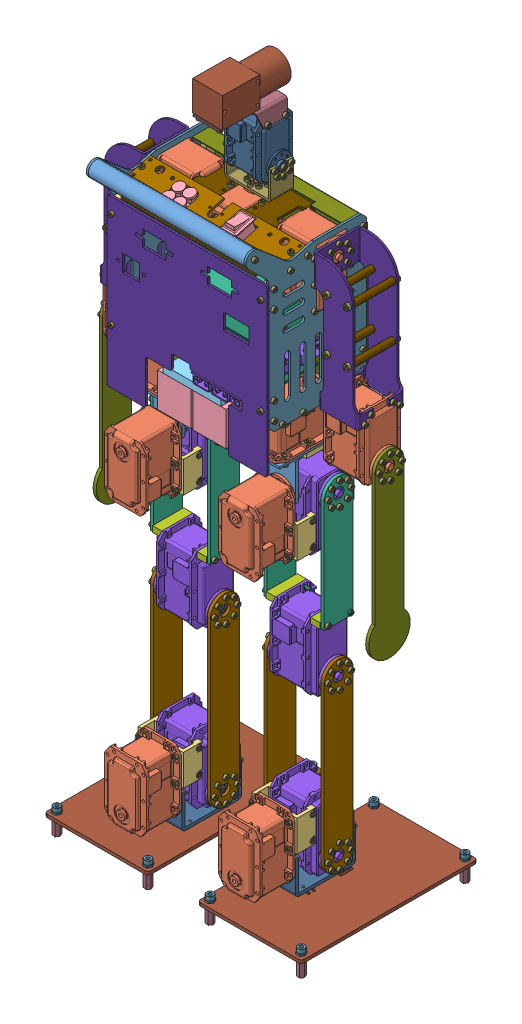
SolidWorks assembly 机器人, configuration 默认. Lengths in mm. (continued)
Components (placement in the parent): (continued)
- 躯干-1: 躯干 [默认] at (1014.3063 415.9938 -67.5657) size (172 287.24 163.85) (continued)
  - hexagon socket head cap screws gb-80: hexagon socket head cap screws gb [GB_FASTENER_SCREWS_HSHCS M2.5X6-N] at (86.3339 35.9855 124.55) x (0 1 0) z (0 0 1) size (8.5 4.5 4.5)
  - hexagon socket head cap screws gb-81: hexagon socket head cap screws gb [GB_FASTENER_SCREWS_HSHCS M2.5X6-N] at (-58.0661 35.9855 124.55) x (0 1 0) z (0 0 1) size (8.5 4.5 4.5)
  - hexagon socket head cap screws gb-82: hexagon socket head cap screws gb [GB_FASTENER_SCREWS_HSHCS M2.5X6-N] at (-58.0661 35.9855 146.55) x (0 1 0) z (0 0 1) size (8.5 4.5 4.5)
  - hexagon socket head cap screws gb-83: hexagon socket head cap screws gb [GB_FASTENER_SCREWS_HSHCS M2.5X6-N] at (-58.0661 35.9855 168.55) x (0 1 0) z (0 0 1) size (8.5 4.5 4.5)
  - hexagon socket head cap screws gb-84: hexagon socket head cap screws gb [GB_FASTENER_SCREWS_HSHCS M2.5X6-N] at (-58.0661 11.9855 124.55) x (0 -1 0) z (0 0 1) size (8.5 4.5 4.5)
  - hexagon socket head cap screws gb-85: hexagon socket head cap screws gb [GB_FASTENER_SCREWS_HSHCS M2.5X6-N] at (-58.0661 11.9855 146.55) x (0 -1 0) z (0 0 1) size (8.5 4.5 4.5)
  - hexagon socket head cap screws gb-86: hexagon socket head cap screws gb [GB_FASTENER_SCREWS_HSHCS M2.5X6-N] at (-58.0661 2.4855 168.55) x (0 1 0) z (0 0 1) size (8.5 4.5 4.5)
  - hexagon socket head cap screws gb-87: hexagon socket head cap screws gb [GB_FASTENER_SCREWS_HSHCS M2.5X6-N] at (-23.4661 2.4855 168.55) x (0 1 0) z (0 0 1) size (8.5 4.5 4.5)
  - hexagon socket head cap screws gb-89: hexagon socket head cap screws gb [GB_FASTENER_SCREWS_HSHCS M2.5X6-N] at (86.3339 11.9855 146.55) x (0 -1 0) z (0 0 1) size (8.5 4.5 4.5)
  - hexagon socket head cap screws gb-90: hexagon socket head cap screws gb [GB_FASTENER_SCREWS_HSHCS M2.5X6-N] at (86.3339 117.6114 168.55) x (0 -1 0) z (0 0 1) size (8.5 4.5 4.5)
  - hexagon socket head cap screws gb-91: hexagon socket head cap screws gb [GB_FASTENER_SCREWS_HSHCS M2.5X6-N] at (86.3339 2.4855 168.55) x (0 1 0) z (0 0 1) size (8.5 4.5 4.5)
  - hexagon socket head cap screws gb-92: hexagon socket head cap screws gb [GB_FASTENER_SCREWS_HSHCS M2.5X6-N] at (-23.4661 11.9855 124.55) x (0 -1 0) z (0 0 1) size (8.5 4.5 4.5)
  - hexagon socket head cap screws gb-93: hexagon socket head cap screws gb [GB_FASTENER_SCREWS_HSHCS M2.5X6-N] at (-23.4661 11.9855 146.55) x (0 -1 0) z (0 0 1) size (8.5 4.5 4.5)
  - hexagon socket head cap screws gb-94: hexagon socket head cap screws gb [GB_FASTENER_SCREWS_HSHCS M2.5X6-N] at (51.7339 11.9855 124.55) x (0 -1 0) z (0 0 1) size (8.5 4.5 4.5)
  - hexagon socket head cap screws gb-95: hexagon socket head cap screws gb [GB_FASTENER_SCREWS_HSHCS M2.5X6-N] at (51.7339 11.9855 146.55) x (0 -1 0) z (0 0 1) size (8.5 4.5 4.5)
  - hexagon socket head cap screws gb-96: hexagon socket head cap screws gb [GB_FASTENER_SCREWS_HSHCS M2.5X6-N] at (50.6339 166.8855 111.25) size (8.5 4.5 4.5)
  - hexagon socket head cap screws gb-97: hexagon socket head cap screws gb [GB_FASTENER_SCREWS_HSHCS M2.5X6-N] at (29.1612 177.7582 116.85) x (0 -1 0) z (0 0 1) size (8.5 4.5 4.5)
  - hexagon socket head cap screws gb-98: hexagon socket head cap screws gb [GB_FASTENER_SCREWS_HSHCS M2.5X6-N] at (-0.8934 177.7582 116.85) x (0 -1 0) z (0 0 1) size (8.5 4.5 4.5)
  - hexagon socket head cap screws gb-99: hexagon socket head cap screws gb [GB_FASTENER_SCREWS_HSHCS M2.5X6-N] at (-22.3661 166.8855 111.25) x (-1 0 0) z (0 0.924225 0.381849) size (8.5 4.5 4.5)
  - hexagon socket head cap screws gb-100: hexagon socket head cap screws gb [GB_FASTENER_SCREWS_HSHCS M2.5X6-N] at (14.1066 184.3582 121.35) x (0 -1 0) z (0 0 1) size (8.5 4.5 4.5)
  - hexagon socket head cap screws gb-101: hexagon socket head cap screws gb [GB_FASTENER_SCREWS_HSHCS M2.5X6-N] at (39.8284 204.3809 121.564) x (-0.999965 0 -0.008321) z (0.008321 0 -0.999965) size (8.5 4.5 4.5)
  - hexagon socket head cap screws gb-102: hexagon socket head cap screws gb [GB_FASTENER_SCREWS_HSHCS M2.5X6-N] at (-8.6199 204.3809 121.1609) x (0.999965 0 0.008321) z (-0.008321 0 0.999965) size (8.5 4.5 4.5)
  - hexagon socket head cap screws gb-103: hexagon socket head cap screws gb [GB_FASTENER_SCREWS_HSHCS M2.5X6-N] at (-0.8934 177.7582 133.85) x (0 -1 0) z (0 0 1) size (8.5 4.5 4.5)
  - hexagon socket head cap screws gb-104: hexagon socket head cap screws gb [GB_FASTENER_SCREWS_HSHCS M2.5X6-N] at (-22.3661 166.8855 145.85) x (-1 0 0) z (0 0.924225 0.381849) size (8.5 4.5 4.5)
  - hexagon socket head cap screws gb-105: hexagon socket head cap screws gb [GB_FASTENER_SCREWS_HSHCS M2.5X6-N] at (50.6339 166.8855 145.85) size (8.5 4.5 4.5)
  - hexagon socket head cap screws gb-106: hexagon socket head cap screws gb [GB_FASTENER_SCREWS_HSHCS M2.5X6-N] at (29.1612 177.7582 133.85) x (0 -1 0) z (0 0 1) size (8.5 4.5 4.5)
  - hexagon socket head cap screws gb-107: hexagon socket head cap screws gb [GB_FASTENER_SCREWS_HSHCS M2.5X6-N] at (8.497 183.5082 115.6463) x (0 -1 0) z (0 0 1) size (8.5 4.5 4.5)
  - hexagon socket head cap screws gb-108: hexagon socket head cap screws gb [GB_FASTENER_SCREWS_HSHCS M2.5X6-N] at (6.1069 183.5082 121.2834) x (0 -1 0) z (0 0 1) size (8.5 4.5 4.5)
  - hexagon socket head cap screws gb-109: hexagon socket head cap screws gb [GB_FASTENER_SCREWS_HSHCS M2.5X6-N] at (8.4029 183.5082 126.9596) x (0 -1 0) z (0 0 1) size (8.5 4.5 4.5)
  - hexagon socket head cap screws gb-110: hexagon socket head cap screws gb [GB_FASTENER_SCREWS_HSHCS M2.5X6-N] at (14.04 183.5082 129.3497) x (0 -1 0) z (0 0 1) size (8.5 4.5 4.5)
  - hexagon socket head cap screws gb-111: hexagon socket head cap screws gb [GB_FASTENER_SCREWS_HSHCS M2.5X6-N] at (19.7162 183.5082 127.0537) x (0 -1 0) z (0 0 1) size (8.5 4.5 4.5)
  - hexagon socket head cap screws gb-112: hexagon socket head cap screws gb [GB_FASTENER_SCREWS_HSHCS M2.5X6-N] at (22.1063 183.5082 121.4166) x (0 -1 0) z (0 0 1) size (8.5 4.5 4.5)
  - hexagon socket head cap screws gb-113: hexagon socket head cap screws gb [GB_FASTENER_SCREWS_HSHCS M2.5X6-N] at (19.8103 183.5082 115.7404) x (0 -1 0) z (0 0 1) size (8.5 4.5 4.5)
  - hexagon socket head cap screws gb-114: hexagon socket head cap screws gb [GB_FASTENER_SCREWS_HSHCS M2.5X6-N] at (14.1732 183.5082 113.3503) x (0 -1 0) z (0 0 1) size (8.5 4.5 4.5)
  - hexagon socket head cap screws gb-115: hexagon socket head cap screws gb [GB_FASTENER_SCREWS_HSHCS M2.5X6-N] at (93.6339 194.6934 203.5985) x (-1 0 0) z (0 0.924225 0.381849) size (8.5 4.5 4.5)
  - hexagon socket head cap screws gb-116: hexagon socket head cap screws gb [GB_FASTENER_SCREWS_HSHCS M2.5X6-N] at (-65.3661 194.6934 203.5985) size (8.5 4.5 4.5)
  - hexagon socket head cap screws gb-117: hexagon socket head cap screws gb [GB_FASTENER_SCREWS_HSHCS M2.5X6-N] at (23.6707 250.2249 136.7301) x (0 1 0) z (-0.004657 0 0.999989) size (8.5 4.5 4.5)
  - hexagon socket head cap screws gb-118: hexagon socket head cap screws gb [GB_FASTENER_SCREWS_HSHCS M2.5X6-N] at (3.6713 250.2249 136.5637) x (0 1 0) z (-0.004657 0 0.999989) size (8.5 4.5 4.5)
  - hexagon socket head cap screws gb-119: hexagon socket head cap screws gb [GB_FASTENER_SCREWS_HSHCS M2.5X6-N] at (3.4076 250.2249 168.2626) x (0 1 0) z (-0.004657 0 0.999989) size (8.5 4.5 4.5)
  - hexagon socket head cap screws gb-120: hexagon socket head cap screws gb [GB_FASTENER_SCREWS_HSHCS M2.5X6-N] at (23.4069 250.2249 168.429) x (0 1 0) z (-0.004657 0 0.999989) size (8.5 4.5 4.5)
  - Back-1: Back [默认] at (14.1339 170.328 166.311) x (1 0 0) z (0 0.965926 0.258819) size (100 30 26.32)
- hexagon socket head cap screws gb-1: hexagon socket head cap screws gb [GB_FASTENER_SCREWS_HSHCS M2.5X6-N] at (1114.4402 589.8793 60.9843) x (-1 0 0) z (0 0.924225 0.381849) size (8.5 4.5 4.5)
- hexagon socket head cap screws gb-2: hexagon socket head cap screws gb [GB_FASTENER_SCREWS_HSHCS M2.5X6-N] at (1114.4402 586.6575 53.2061) x (-1 0 0) z (0 0.924225 0.381849) size (8.5 4.5 4.5)
- hexagon socket head cap screws gb-3: hexagon socket head cap screws gb [GB_FASTENER_SCREWS_HSHCS M2.5X6-N] at (1114.4402 578.8793 49.9843) x (-1 0 0) z (0 0.924225 0.381849) size (8.5 4.5 4.5)
- hexagon socket head cap screws gb-4: hexagon socket head cap screws gb [GB_FASTENER_SCREWS_HSHCS M2.5X6-N] at (1114.4402 571.1012 53.2061) x (-1 0 0) z (0 0.924225 0.381849) size (8.5 4.5 4.5)
- hexagon socket head cap screws gb-5: hexagon socket head cap screws gb [GB_FASTENER_SCREWS_HSHCS M2.5X6-N] at (1114.4402 567.8793 60.9843) x (-1 0 0) z (0 0.924225 0.381849) size (8.5 4.5 4.5)
- hexagon socket head cap screws gb-6: hexagon socket head cap screws gb [GB_FASTENER_SCREWS_HSHCS M2.5X6-N] at (1114.4402 571.1012 68.7625) x (-1 0 0) z (0 0.924225 0.381849) size (8.5 4.5 4.5)
- hexagon socket head cap screws gb-7: hexagon socket head cap screws gb [GB_FASTENER_SCREWS_HSHCS M2.5X6-N] at (1114.4402 578.8793 71.9843) x (-1 0 0) z (0 0.924225 0.381849) size (8.5 4.5 4.5)
- hexagon socket head cap screws gb-8: hexagon socket head cap screws gb [GB_FASTENER_SCREWS_HSHCS M2.5X6-N] at (1114.4402 586.6575 68.7625) x (-1 0 0) z (0 0.924225 0.381849) size (8.5 4.5 4.5)
- hexagon socket head cap screws gb-25: hexagon socket head cap screws gb [GB_FASTENER_SCREWS_HSHCS M2.5X6-N] at (942.4402 586.6575 68.7625) size (8.5 4.5 4.5)
- hexagon socket head cap screws gb-26: hexagon socket head cap screws gb [GB_FASTENER_SCREWS_HSHCS M2.5X6-N] at (942.4402 578.8793 71.9843) size (8.5 4.5 4.5)
- hexagon socket head cap screws gb-27: hexagon socket head cap screws gb [GB_FASTENER_SCREWS_HSHCS M2.5X6-N] at (942.4402 571.1012 68.7625) size (8.5 4.5 4.5)
- hexagon socket head cap screws gb-28: hexagon socket head cap screws gb [GB_FASTENER_SCREWS_HSHCS M2.5X6-N] at (942.4402 567.8793 60.9843) size (8.5 4.5 4.5)
- hexagon socket head cap screws gb-29: hexagon socket head cap screws gb [GB_FASTENER_SCREWS_HSHCS M2.5X6-N] at (942.4402 589.8793 60.9843) size (8.5 4.5 4.5)
- hexagon socket head cap screws gb-30: hexagon socket head cap screws gb [GB_FASTENER_SCREWS_HSHCS M2.5X6-N] at (942.4402 586.6575 53.2061) size (8.5 4.5 4.5)
- hexagon socket head cap screws gb-31: hexagon socket head cap screws gb [GB_FASTENER_SCREWS_HSHCS M2.5X6-N] at (942.4402 578.8793 49.9843) size (8.5 4.5 4.5)
- hexagon socket head cap screws gb-32: hexagon socket head cap screws gb [GB_FASTENER_SCREWS_HSHCS M2.5X6-N] at (942.4402 571.1012 53.2061) size (8.5 4.5 4.5)
- hexagon socket head cap screws gb-49: hexagon socket head cap screws gb [GB_FASTENER_SCREWS_HSHCS M2.5X6-N] at (965.762 410.9793 53.2061) x (0 1 0) z (0 0 1) size (8.5 4.5 4.5)
- hexagon socket head cap screws gb-50: hexagon socket head cap screws gb [GB_FASTENER_SCREWS_HSHCS M2.5X6-N] at (962.5402 410.9793 60.9843) x (0 1 0) z (0 0 1) size (8.5 4.5 4.5)
- hexagon socket head cap screws gb-51: hexagon socket head cap screws gb [GB_FASTENER_SCREWS_HSHCS M2.5X6-N] at (965.762 410.9793 68.7625) x (0 1 0) z (0 0 1) size (8.5 4.5 4.5)
- hexagon socket head cap screws gb-52: hexagon socket head cap screws gb [GB_FASTENER_SCREWS_HSHCS M2.5X6-N] at (973.5402 410.9793 71.9843) x (0 1 0) z (0 0 1) size (8.5 4.5 4.5)
- hexagon socket head cap screws gb-53: hexagon socket head cap screws gb [GB_FASTENER_SCREWS_HSHCS M2.5X6-N] at (981.3184 410.9793 68.7625) x (0 1 0) z (0 0 1) size (8.5 4.5 4.5)
- hexagon socket head cap screws gb-54: hexagon socket head cap screws gb [GB_FASTENER_SCREWS_HSHCS M2.5X6-N] at (981.3184 410.9793 53.2061) x (0 1 0) z (0 0 1) size (8.5 4.5 4.5)
- hexagon socket head cap screws gb-55: hexagon socket head cap screws gb [GB_FASTENER_SCREWS_HSHCS M2.5X6-N] at (973.5402 410.9793 49.9843) x (0 1 0) z (0 0 1) size (8.5 4.5 4.5)
- hexagon socket head cap screws gb-56: hexagon socket head cap screws gb [GB_FASTENER_SCREWS_HSHCS M2.5X6-N] at (984.5402 410.9793 60.9843) x (0 1 0) z (0 0 1) size (8.5 4.5 4.5)
- hexagon socket head cap screws gb-57: hexagon socket head cap screws gb [GB_FASTENER_SCREWS_HSHCS M2.5X6-N] at (1094.3402 410.9793 60.9843) x (0 1 0) z (0 0 1) size (8.5 4.5 4.5)
- hexagon socket head cap screws gb-58: hexagon socket head cap screws gb [GB_FASTENER_SCREWS_HSHCS M2.5X6-N] at (1091.1184 410.9793 53.2061) x (0 1 0) z (0 0 1) size (8.5 4.5 4.5)
- hexagon socket head cap screws gb-59: hexagon socket head cap screws gb [GB_FASTENER_SCREWS_HSHCS M2.5X6-N] at (1083.3402 410.9793 49.9843) x (0 1 0) z (0 0 1) size (8.5 4.5 4.5)
- hexagon socket head cap screws gb-60: hexagon socket head cap screws gb [GB_FASTENER_SCREWS_HSHCS M2.5X6-N] at (1075.562 410.9793 53.2061) x (0 1 0) z (0 0 1) size (8.5 4.5 4.5)
- hexagon socket head cap screws gb-61: hexagon socket head cap screws gb [GB_FASTENER_SCREWS_HSHCS M2.5X6-N] at (1072.3402 410.9793 60.9843) x (0 1 0) z (0 0 1) size (8.5 4.5 4.5)
- hexagon socket head cap screws gb-62: hexagon socket head cap screws gb [GB_FASTENER_SCREWS_HSHCS M2.5X6-N] at (1091.1184 410.9793 68.7625) x (0 1 0) z (0 0 1) size (8.5 4.5 4.5)
- hexagon socket head cap screws gb-63: hexagon socket head cap screws gb [GB_FASTENER_SCREWS_HSHCS M2.5X6-N] at (1083.3402 410.9793 71.9843) x (0 1 0) z (0 0 1) size (8.5 4.5 4.5)
- hexagon socket head cap screws gb-64: hexagon socket head cap screws gb [GB_FASTENER_SCREWS_HSHCS M2.5X6-N] at (1075.562 410.9793 68.7625) x (0 1 0) z (0 0 1) size (8.5 4.5 4.5)
- hexagon socket head cap screws gb-65: hexagon socket head cap screws gb [GB_FASTENER_SCREWS_HSHCS M2.5X6-N] at (1091.1184 410.9793 53.2061) x (0 1 0) z (0 0 1) size (8.5 4.5 4.5)
- hexagon socket head cap screws gb-66: hexagon socket head cap screws gb [GB_FASTENER_SCREWS_HSHCS M2.5X6-N] at (1094.3402 410.9793 60.9843) x (0 1 0) z (0 0 1) size (8.5 4.5 4.5)
- hexagon socket head cap screws gb-67: hexagon socket head cap screws gb [GB_FASTENER_SCREWS_HSHCS M2.5X6-N] at (1091.1184 410.9793 68.7625) x (0 1 0) z (0 0 1) size (8.5 4.5 4.5)
- hexagon socket head cap screws gb-68: hexagon socket head cap screws gb [GB_FASTENER_SCREWS_HSHCS M2.5X6-N] at (1083.3402 410.9793 71.9843) x (0 1 0) z (0 0 1) size (8.5 4.5 4.5)
- hexagon socket head cap screws gb-69: hexagon socket head cap screws gb [GB_FASTENER_SCREWS_HSHCS M2.5X6-N] at (1075.562 410.9793 68.7625) x (0 1 0) z (0 0 1) size (8.5 4.5 4.5)
- hexagon socket head cap screws gb-70: hexagon socket head cap screws gb [GB_FASTENER_SCREWS_HSHCS M2.5X6-N] at (1072.3402 410.9793 60.9843) x (0 1 0) z (0 0 1) size (8.5 4.5 4.5)
- hexagon socket head cap screws gb-71: hexagon socket head cap screws gb [GB_FASTENER_SCREWS_HSHCS M2.5X6-N] at (1075.562 410.9793 53.2061) x (0 1 0) z (0 0 1) size (8.5 4.5 4.5)
- hexagon socket head cap screws gb-72: hexagon socket head cap screws gb [GB_FASTENER_SCREWS_HSHCS M2.5X6-N] at (1083.3402 410.9793 49.9843) x (0 1 0) z (0 0 1) size (8.5 4.5 4.5)
- hexagon socket head cap screws gb-73: hexagon socket head cap screws gb [GB_FASTENER_SCREWS_HSHCS M2.5X6-N] at (973.5402 410.9793 49.9843) x (0 1 0) z (0 0 1) size (8.5 4.5 4.5)
- hexagon socket head cap screws gb-74: hexagon socket head cap screws gb [GB_FASTENER_SCREWS_HSHCS M2.5X6-N] at (981.3184 410.9793 53.2061) x (0 1 0) z (0 0 1) size (8.5 4.5 4.5)
- hexagon socket head cap screws gb-75: hexagon socket head cap screws gb [GB_FASTENER_SCREWS_HSHCS M2.5X6-N] at (984.5402 410.9793 60.9843) x (0 1 0) z (0 0 1) size (8.5 4.5 4.5)
- hexagon socket head cap screws gb-76: hexagon socket head cap screws gb [GB_FASTENER_SCREWS_HSHCS M2.5X6-N] at (981.3184 410.9793 68.7625) x (0 1 0) z (0 0 1) size (8.5 4.5 4.5)
- hexagon socket head cap screws gb-77: hexagon socket head cap screws gb [GB_FASTENER_SCREWS_HSHCS M2.5X6-N] at (973.5402 410.9793 71.9843) x (0 1 0) z (0 0 1) size (8.5 4.5 4.5)
- hexagon socket head cap screws gb-78: hexagon socket head cap screws gb [GB_FASTENER_SCREWS_HSHCS M2.5X6-N] at (965.762 410.9793 68.7625) x (0 1 0) z (0 0 1) size (8.5 4.5 4.5)
- hexagon socket head cap screws gb-79: hexagon socket head cap screws gb [GB_FASTENER_SCREWS_HSHCS M2.5X6-N] at (962.5402 410.9793 60.9843) x (0 1 0) z (0 0 1) size (8.5 4.5 4.5)
- hexagon socket head cap screws gb-80: hexagon socket head cap screws gb [GB_FASTENER_SCREWS_HSHCS M2.5X6-N] at (965.762 410.9793 53.2061) x (0 1 0) z (0 0 1) size (8.5 4.5 4.5)
- hexagon socket head cap screws gb-81: hexagon socket head cap screws gb [GB_FASTENER_SCREWS_HSHCS M2.5X8-N] at (1155.9856 467.8793 44.0843) x (-1 0 0) z (0 0.924225 0.381849) size (10.5 4.5 4.5)
- hexagon socket head cap screws gb-82: hexagon socket head cap screws gb [GB_FASTENER_SCREWS_HSHCS M2.5X8-N] at (1155.9856 473.1793 50.3843) x (-1 0 0) z (0 0.924225 0.381849) size (10.5 4.5 4.5)
- hexagon socket head cap screws gb-83: hexagon socket head cap screws gb [GB_FASTENER_SCREWS_HSHCS M2.5X8-N] at (1155.9856 473.1793 71.5843) x (-1 0 0) z (0 0.924225 0.381849) size (10.5 4.5 4.5)
- hexagon socket head cap screws gb-84: hexagon socket head cap screws gb [GB_FASTENER_SCREWS_HSHCS M2.5X8-N] at (1155.9856 467.8793 77.8843) x (-1 0 0) z (0 0.924225 0.381849) size (10.5 4.5 4.5)
- hexagon socket head cap screws gb-85: hexagon socket head cap screws gb [GB_FASTENER_SCREWS_HSHCS M2.5X8-N] at (1112.6402 467.8793 44.0843) size (10.5 4.5 4.5)
- hexagon socket head cap screws gb-86: hexagon socket head cap screws gb [GB_FASTENER_SCREWS_HSHCS M2.5X8-N] at (1112.6402 473.1793 50.3843) size (10.5 4.5 4.5)
- hexagon socket head cap screws gb-87: hexagon socket head cap screws gb [GB_FASTENER_SCREWS_HSHCS M2.5X8-N] at (1112.6402 473.1793 71.5843) size (10.5 4.5 4.5)
- hexagon socket head cap screws gb-88: hexagon socket head cap screws gb [GB_FASTENER_SCREWS_HSHCS M2.5X8-N] at (1112.6402 467.8793 77.8843) size (10.5 4.5 4.5)
- hexagon socket head cap screws gb-89: hexagon socket head cap screws gb [GB_FASTENER_SCREWS_HSHCS M2.5X8-N] at (900.8949 473.1793 71.5843) size (10.5 4.5 4.5)
- hexagon socket head cap screws gb-90: hexagon socket head cap screws gb [GB_FASTENER_SCREWS_HSHCS M2.5X8-N] at (900.8949 467.8793 77.8843) size (10.5 4.5 4.5)
- hexagon socket head cap screws gb-91: hexagon socket head cap screws gb [GB_FASTENER_SCREWS_HSHCS M2.5X8-N] at (900.8949 473.1793 50.3843) size (10.5 4.5 4.5)
- hexagon socket head cap screws gb-92: hexagon socket head cap screws gb [GB_FASTENER_SCREWS_HSHCS M2.5X8-N] at (900.8949 467.8793 44.0843) size (10.5 4.5 4.5)
- hexagon socket head cap screws gb-93: hexagon socket head cap screws gb [GB_FASTENER_SCREWS_HSHCS M2.5X8-N] at (944.2402 473.1793 71.5843) x (-1 0 0) z (0 0.924225 0.381849) size (10.5 4.5 4.5)
- hexagon socket head cap screws gb-94: hexagon socket head cap screws gb [GB_FASTENER_SCREWS_HSHCS M2.5X8-N] at (944.2402 467.8793 77.8843) x (-1 0 0) z (0 0.924225 0.381849) size (10.5 4.5 4.5)
- hexagon socket head cap screws gb-95: hexagon socket head cap screws gb [GB_FASTENER_SCREWS_HSHCS M2.5X8-N] at (944.2402 473.1793 50.3843) x (-1 0 0) z (0 0.924225 0.381849) size (10.5 4.5 4.5)
- hexagon socket head cap screws gb-96: hexagon socket head cap screws gb [GB_FASTENER_SCREWS_HSHCS M2.5X8-N] at (944.2402 467.8793 44.0843) x (-1 0 0) z (0 0.924225 0.381849) size (10.5 4.5 4.5)
- hexagon socket head cap screws gb-97: hexagon socket head cap screws gb [GB_FASTENER_SCREWS_HSHCS M3X6-N] at (1124.3129 564.8793 35.6116) x (0 0 1) z (-1 0 0) size (9 5.5 5.5)
- hexagon socket head cap screws gb-98: hexagon socket head cap screws gb [GB_FASTENER_SCREWS_HSHCS M3X6-N] at (1144.3129 564.8793 35.6116) x (0 0 1) z (-1 0 0) size (9 5.5 5.5)
- hexagon socket head cap screws gb-99: hexagon socket head cap screws gb [GB_FASTENER_SCREWS_HSHCS M3X6-N] at (1144.3129 514.8793 35.6116) x (0 0 1) z (-1 0 0) size (9 5.5 5.5)
- hexagon socket head cap screws gb-100: hexagon socket head cap screws gb [GB_FASTENER_SCREWS_HSHCS M3X6-N] at (1124.3129 514.8793 35.6116) x (0 0 1) z (-1 0 0) size (9 5.5 5.5)
- hexagon socket head cap screws gb-101: hexagon socket head cap screws gb [GB_FASTENER_SCREWS_HSHCS M3X6-N] at (1124.3129 564.8793 86.357) x (0 0 -1) z (1 0 0) size (9 5.5 5.5)
- hexagon socket head cap screws gb-102: hexagon socket head cap screws gb [GB_FASTENER_SCREWS_HSHCS M3X6-N] at (1144.3129 564.8793 86.357) x (0 0 -1) z (1 0 0) size (9 5.5 5.5)
- hexagon socket head cap screws gb-103: hexagon socket head cap screws gb [GB_FASTENER_SCREWS_HSHCS M3X6-N] at (1124.3129 514.8793 86.357) x (0 0 -1) z (1 0 0) size (9 5.5 5.5)
- hexagon socket head cap screws gb-104: hexagon socket head cap screws gb [GB_FASTENER_SCREWS_HSHCS M3X6-N] at (1144.3129 514.8793 86.357) x (0 0 -1) z (1 0 0) size (9 5.5 5.5)
- hexagon socket head cap screws gb-105: hexagon socket head cap screws gb [GB_FASTENER_SCREWS_HSHCS M3X6-N] at (912.5675 514.8793 86.357) x (0 0 -1) z (1 0 0) size (9 5.5 5.5)
- hexagon socket head cap screws gb-107: hexagon socket head cap screws gb [GB_FASTENER_SCREWS_HSHCS M3X6-N] at (912.5675 564.8793 86.357) x (0 0 -1) z (1 0 0) size (9 5.5 5.5)
- hexagon socket head cap screws gb-108: hexagon socket head cap screws gb [GB_FASTENER_SCREWS_HSHCS M3X6-N] at (932.5675 564.8793 86.357) x (0 0 -1) z (1 0 0) size (9 5.5 5.5)
- hexagon socket head cap screws gb-109: hexagon socket head cap screws gb [GB_FASTENER_SCREWS_HSHCS M3X6-N] at (932.5675 514.8793 86.357) x (0 0 -1) z (1 0 0) size (9 5.5 5.5)
- hexagon socket head cap screws gb-110: hexagon socket head cap screws gb [GB_FASTENER_SCREWS_HSHCS M3X6-N] at (932.5675 564.8793 35.6116) x (0 0 1) z (-1 0 0) size (9 5.5 5.5)
- hexagon socket head cap screws gb-111: hexagon socket head cap screws gb [GB_FASTENER_SCREWS_HSHCS M3X6-N] at (912.5675 564.8793 35.6116) x (0 0 1) z (-1 0 0) size (9 5.5 5.5)
- hexagon socket head cap screws gb-112: hexagon socket head cap screws gb [GB_FASTENER_SCREWS_HSHCS M3X6-N] at (932.5675 514.8793 35.6116) x (0 0 1) z (-1 0 0) size (9 5.5 5.5)
- hexagon socket head cap screws gb-113: hexagon socket head cap screws gb [GB_FASTENER_SCREWS_HSHCS M3X6-N] at (912.5675 514.8793 35.6116) x (0 0 1) z (-1 0 0) size (9 5.5 5.5)
Mates (geometry in assembly coordinates):
- 同心5: concentric: cylinder of assembly; cylinder of assembly; cylinder of 手臂-2/机器人-上臂骨-1 through (1109.9402 589.8793 60.9843) axis (1 0 0) radius 1.35; cylinder of hexagon socket head cap screws gb-1 through (1105.9402 589.8793 60.9843) axis (1 0 0) radius 1.25
- 重合11: coincident: plane of assembly; plane of assembly; plane of 手臂-2/机器人-上臂骨-1 through (1111.9402 564.8793 90.9843) normal (1 0 0); plane of hexagon socket head cap screws gb-1 through (1111.9402 589.8793 60.9843) normal (-1 0 0)
- 同心6: concentric: cylinder of assembly; cylinder of assembly; cylinder of 手臂-2/机器人-上臂骨-1 through (1109.9402 586.6575 53.2061) axis (1 0 0) radius 1.35; cylinder of hexagon socket head cap screws gb-2 through (1105.9402 586.6575 53.2061) axis (1 0 0) radius 1.25
- 重合12: coincident: plane of assembly; plane of assembly; plane of 手臂-2/机器人-上臂骨-1 through (1111.9402 564.8793 90.9843) normal (1 0 0); plane of hexagon socket head cap screws gb-2 through (1111.9402 586.6575 53.2061) normal (-1 0 0)
- 同心7: concentric: cylinder of assembly; cylinder of assembly; cylinder of 手臂-2/机器人-上臂骨-1 through (1109.9402 578.8793 49.9843) axis (1 0 0) radius 1.35; cylinder of hexagon socket head cap screws gb-3 through (1105.9402 578.8793 49.9843) axis (1 0 0) radius 1.25
- 重合13: coincident: plane of assembly; plane of assembly; plane of 手臂-2/机器人-上臂骨-1 through (1111.9402 564.8793 90.9843) normal (1 0 0); plane of hexagon socket head cap screws gb-3 through (1111.9402 578.8793 49.9843) normal (-1 0 0)
- 同心8: concentric: cylinder of assembly; cylinder of assembly; cylinder of 手臂-2/机器人-上臂骨-1 through (1109.9402 571.1012 53.2061) axis (1 0 0) radius 1.35; cylinder of hexagon socket head cap screws gb-4 through (1105.9402 571.1012 53.2061) axis (1 0 0) radius 1.25
- 重合14: coincident: plane of assembly; plane of assembly; plane of 手臂-2/机器人-上臂骨-1 through (1111.9402 564.8793 90.9843) normal (1 0 0); plane of hexagon socket head cap screws gb-4 through (1111.9402 571.1012 53.2061) normal (-1 0 0)
- 同心9: concentric: cylinder of assembly; cylinder of assembly; cylinder of 手臂-2/机器人-上臂骨-1 through (1109.9402 567.8793 60.9843) axis (1 0 0) radius 1.35; cylinder of hexagon socket head cap screws gb-5 through (1105.9402 567.8793 60.9843) axis (1 0 0) radius 1.25
- 重合15: coincident: plane of assembly; plane of assembly; plane of 手臂-2/机器人-上臂骨-1 through (1111.9402 564.8793 90.9843) normal (1 0 0); plane of hexagon socket head cap screws gb-5 through (1111.9402 567.8793 60.9843) normal (-1 0 0)
- 同心10: concentric: cylinder of assembly; cylinder of assembly; cylinder of 手臂-2/机器人-上臂骨-1 through (1109.9402 571.1012 68.7625) axis (1 0 0) radius 1.35; cylinder of hexagon socket head cap screws gb-6 through (1105.9402 571.1012 68.7625) axis (1 0 0) radius 1.25
- 重合16: coincident: plane of assembly; plane of assembly; plane of 手臂-2/机器人-上臂骨-1 through (1111.9402 564.8793 90.9843) normal (1 0 0); plane of hexagon socket head cap screws gb-6 through (1111.9402 571.1012 68.7625) normal (-1 0 0)
- 同心11: concentric: cylinder of assembly; cylinder of assembly; cylinder of 手臂-2/机器人-上臂骨-1 through (1109.9402 578.8793 71.9843) axis (1 0 0) radius 1.35; cylinder of hexagon socket head cap screws gb-7 through (1105.9402 578.8793 71.9843) axis (1 0 0) radius 1.25
- 重合17: coincident: plane of assembly; plane of assembly; plane of 手臂-2/机器人-上臂骨-1 through (1111.9402 564.8793 90.9843) normal (1 0 0); plane of hexagon socket head cap screws gb-7 through (1111.9402 578.8793 71.9843) normal (-1 0 0)
- 同心12: concentric: cylinder of assembly; cylinder of assembly; cylinder of 手臂-2/机器人-上臂骨-1 through (1109.9402 586.6575 68.7625) axis (1 0 0) radius 1.35; cylinder of hexagon socket head cap screws gb-8 through (1105.9402 586.6575 68.7625) axis (1 0 0) radius 1.25
- 重合18: coincident: plane of assembly; plane of assembly; plane of 手臂-2/机器人-上臂骨-1 through (1111.9402 564.8793 90.9843) normal (1 0 0); plane of hexagon socket head cap screws gb-8 through (1111.9402 586.6575 68.7625) normal (-1 0 0)
- 同心29: concentric: cylinder of assembly; cylinder of assembly; cylinder of 手臂-1/机器人-上臂骨-1 through (946.9402 586.6575 68.7625) axis (-1 0 0) radius 1.35; cylinder of hexagon socket head cap screws gb-25 through (950.9402 586.6575 68.7625) axis (-1 0 0) radius 1.25
- 重合35: coincident: plane of assembly; plane of assembly; plane of 手臂-1/机器人-上臂骨-1 through (944.9402 564.8793 30.9843) normal (-1 0 0); plane of hexagon socket head cap screws gb-25 through (944.9402 586.6575 68.7625) normal (1 0 0)
- 同心30: concentric: cylinder of assembly; cylinder of assembly; cylinder of 手臂-1/机器人-上臂骨-1 through (946.9402 578.8793 71.9843) axis (-1 0 0) radius 1.35; cylinder of hexagon socket head cap screws gb-26 through (950.9402 578.8793 71.9843) axis (-1 0 0) radius 1.25
- 重合36: coincident: plane of assembly; plane of assembly; plane of 手臂-1/机器人-上臂骨-1 through (944.9402 564.8793 30.9843) normal (-1 0 0); plane of hexagon socket head cap screws gb-26 through (944.9402 578.8793 71.9843) normal (1 0 0)
- 同心31: concentric: cylinder of assembly; cylinder of assembly; cylinder of 手臂-1/机器人-上臂骨-1 through (946.9402 571.1012 68.7625) axis (-1 0 0) radius 1.35; cylinder of hexagon socket head cap screws gb-27 through (950.9402 571.1012 68.7625) axis (-1 0 0) radius 1.25
- 重合37: coincident: plane of assembly; plane of assembly; plane of 手臂-1/机器人-上臂骨-1 through (944.9402 564.8793 30.9843) normal (-1 0 0); plane of hexagon socket head cap screws gb-27 through (944.9402 571.1012 68.7625) normal (1 0 0)
- 同心32: concentric: cylinder of assembly; cylinder of assembly; cylinder of 手臂-1/机器人-上臂骨-1 through (946.9402 567.8793 60.9843) axis (-1 0 0) radius 1.35; cylinder of hexagon socket head cap screws gb-28 through (950.9402 567.8793 60.9843) axis (-1 0 0) radius 1.25
- 重合38: coincident: plane of assembly; plane of assembly; plane of 手臂-1/机器人-上臂骨-1 through (944.9402 564.8793 30.9843) normal (-1 0 0); plane of hexagon socket head cap screws gb-28 through (944.9402 567.8793 60.9843) normal (1 0 0)
- 同心33: concentric: cylinder of assembly; cylinder of assembly; cylinder of 手臂-1/机器人-上臂骨-1 through (946.9402 589.8793 60.9843) axis (-1 0 0) radius 1.35; cylinder of hexagon socket head cap screws gb-29 through (950.9402 589.8793 60.9843) axis (-1 0 0) radius 1.25
- 重合39: coincident: plane of assembly; plane of assembly; plane of 手臂-1/机器人-上臂骨-1 through (944.9402 564.8793 30.9843) normal (-1 0 0); plane of hexagon socket head cap screws gb-29 through (944.9402 589.8793 60.9843) normal (1 0 0)
- 同心34: concentric: cylinder of assembly; cylinder of assembly; cylinder of 手臂-1/机器人-上臂骨-1 through (946.9402 586.6575 53.2061) axis (-1 0 0) radius 1.35; cylinder of hexagon socket head cap screws gb-30 through (950.9402 586.6575 53.2061) axis (-1 0 0) radius 1.25
- 重合40: coincident: plane of assembly; plane of assembly; plane of 手臂-1/机器人-上臂骨-1 through (944.9402 564.8793 30.9843) normal (-1 0 0); plane of hexagon socket head cap screws gb-30 through (944.9402 586.6575 53.2061) normal (1 0 0)
- 同心35: concentric: cylinder of assembly; cylinder of assembly; cylinder of 手臂-1/机器人-上臂骨-1 through (946.9402 578.8793 49.9843) axis (-1 0 0) radius 1.35; cylinder of hexagon socket head cap screws gb-31 through (950.9402 578.8793 49.9843) axis (-1 0 0) radius 1.25
- 重合41: coincident: plane of assembly; plane of assembly; plane of 手臂-1/机器人-上臂骨-1 through (944.9402 564.8793 30.9843) normal (-1 0 0); plane of hexagon socket head cap screws gb-31 through (944.9402 578.8793 49.9843) normal (1 0 0)
- 同心36: concentric: cylinder of assembly; cylinder of assembly; cylinder of 手臂-1/机器人-上臂骨-1 through (946.9402 571.1012 53.2061) axis (-1 0 0) radius 1.35; cylinder of hexagon socket head cap screws gb-32 through (950.9402 571.1012 53.2061) axis (-1 0 0) radius 1.25
- 重合42: coincident: plane of assembly; plane of assembly; plane of 手臂-1/机器人-上臂骨-1 through (944.9402 564.8793 30.9843) normal (-1 0 0); plane of hexagon socket head cap screws gb-32 through (944.9402 571.1012 53.2061) normal (1 0 0)
- 同心53: concentric: cylinder of 左腿-1/机器人-髋关节连接件-1 through (965.762 416.4793 53.2061) axis (0 -1 0) radius 1.35; cylinder of ? through (965.762 419.4793 53.2061) axis (0 -1 0) radius 1.25
- 重合59: coincident: plane of 左腿-1/机器人-髋关节连接件-1 through (973.5402 413.4793 60.9843) normal (0 -1 0); plane of ? through (965.762 413.4793 53.2061) normal (0 1 0)
- 同心54: concentric: cylinder of 左腿-1/机器人-髋关节连接件-1 through (962.5402 416.4793 60.9843) axis (0 -1 0) radius 1.35; cylinder of ? through (962.5402 419.4793 60.9843) axis (0 -1 0) radius 1.25
- 重合60: coincident: plane of 左腿-1/机器人-髋关节连接件-1 through (973.5402 413.4793 60.9843) normal (0 -1 0); plane of ? through (962.5402 413.4793 60.9843) normal (0 1 0)
- 同心55: concentric: cylinder of 左腿-1/机器人-髋关节连接件-1 through (965.762 416.4793 68.7625) axis (0 -1 0) radius 1.35; cylinder of ? through (965.762 419.4793 68.7625) axis (0 -1 0) radius 1.25
- 重合61: coincident: plane of 左腿-1/机器人-髋关节连接件-1 through (973.5402 413.4793 60.9843) normal (0 -1 0); plane of ? through (965.762 413.4793 68.7625) normal (0 1 0)
- 同心56: concentric: cylinder of 左腿-1/机器人-髋关节连接件-1 through (973.5402 416.4793 71.9843) axis (0 -1 0) radius 1.35; cylinder of ? through (973.5402 419.4793 71.9843) axis (0 -1 0) radius 1.25
- 重合62: coincident: plane of 左腿-1/机器人-髋关节连接件-1 through (973.5402 413.4793 60.9843) normal (0 -1 0); plane of ? through (973.5402 413.4793 71.9843) normal (0 1 0)
- 同心57: concentric: cylinder of 左腿-1/机器人-髋关节连接件-1 through (981.3184 416.4793 68.7625) axis (0 -1 0) radius 1.35; cylinder of ? through (981.3184 419.4793 68.7625) axis (0 -1 0) radius 1.25
- 重合63: coincident: plane of 左腿-1/机器人-髋关节连接件-1 through (973.5402 413.4793 60.9843) normal (0 -1 0); plane of ? through (981.3184 413.4793 68.7625) normal (0 1 0)
- 同心58: concentric: cylinder of 左腿-1/机器人-髋关节连接件-1 through (981.3184 416.4793 53.2061) axis (0 -1 0) radius 1.35; cylinder of ? through (981.3184 419.4793 53.2061) axis (0 -1 0) radius 1.25
- 重合64: coincident: plane of 左腿-1/机器人-髋关节连接件-1 through (973.5402 413.4793 60.9843) normal (0 -1 0); plane of ? through (981.3184 413.4793 53.2061) normal (0 1 0)
- 同心59: concentric: cylinder of 左腿-1/机器人-髋关节连接件-1 through (973.5402 416.4793 49.9843) axis (0 -1 0) radius 1.35; cylinder of ? through (973.5402 419.4793 49.9843) axis (0 -1 0) radius 1.25
- 重合65: coincident: plane of 左腿-1/机器人-髋关节连接件-1 through (973.5402 413.4793 60.9843) normal (0 -1 0); plane of ? through (973.5402 413.4793 49.9843) normal (0 1 0)
- 同心60: concentric: cylinder of 左腿-1/机器人-髋关节连接件-1 through (984.5402 416.4793 60.9843) axis (0 -1 0) radius 1.35; cylinder of ? through (984.5402 419.4793 60.9843) axis (0 -1 0) radius 1.25
- 重合66: coincident: plane of 左腿-1/机器人-髋关节连接件-1 through (973.5402 413.4793 60.9843) normal (0 -1 0); plane of ? through (984.5402 413.4793 60.9843) normal (0 1 0)
- 同心61: concentric: cylinder of 右腿-1/机器人-髋关节连接件-1 through (1094.3402 416.4793 60.9843) axis (0 -1 0) radius 1.35; cylinder of ? through (1094.3402 419.4793 60.9843) axis (0 -1 0) radius 1.25
- 重合67: coincident: plane of 右腿-1/机器人-髋关节连接件-1 through (1083.3402 413.4793 60.9843) normal (0 -1 0); plane of ? through (1094.3402 413.4793 60.9843) normal (0 1 0)
- 同心62: concentric: cylinder of 右腿-1/机器人-髋关节连接件-1 through (1091.1184 416.4793 53.2061) axis (0 -1 0) radius 1.35; cylinder of ? through (1091.1184 419.4793 53.2061) axis (0 -1 0) radius 1.25
- 重合68: coincident: plane of 右腿-1/机器人-髋关节连接件-1 through (1083.3402 413.4793 60.9843) normal (0 -1 0); plane of ? through (1091.1184 413.4793 53.2061) normal (0 1 0)
- 同心63: concentric: cylinder of 右腿-1/机器人-髋关节连接件-1 through (1083.3402 416.4793 49.9843) axis (0 -1 0) radius 1.35; cylinder of ? through (1083.3402 419.4793 49.9843) axis (0 -1 0) radius 1.25
- 重合69: coincident: plane of 右腿-1/机器人-髋关节连接件-1 through (1083.3402 413.4793 60.9843) normal (0 -1 0); plane of ? through (1083.3402 413.4793 49.9843) normal (0 1 0)
- 同心64: concentric: cylinder of 右腿-1/机器人-髋关节连接件-1 through (1075.562 416.4793 53.2061) axis (0 -1 0) radius 1.35; cylinder of ? through (1075.562 419.4793 53.2061) axis (0 -1 0) radius 1.25
- 重合70: coincident: plane of 右腿-1/机器人-髋关节连接件-1 through (1083.3402 413.4793 60.9843) normal (0 -1 0); plane of ? through (1075.562 413.4793 53.2061) normal (0 1 0)
- 同心65: concentric: cylinder of 右腿-1/机器人-髋关节连接件-1 through (1072.3402 416.4793 60.9843) axis (0 -1 0) radius 1.35; cylinder of ? through (1072.3402 419.4793 60.9843) axis (0 -1 0) radius 1.25
- 重合71: coincident: plane of 右腿-1/机器人-髋关节连接件-1 through (1083.3402 413.4793 60.9843) normal (0 -1 0); plane of ? through (1072.3402 413.4793 60.9843) normal (0 1 0)
- 同心66: concentric: cylinder of 右腿-1/机器人-髋关节连接件-1 through (1091.1184 416.4793 68.7625) axis (0 -1 0) radius 1.35; cylinder of ? through (1091.1184 419.4793 68.7625) axis (0 -1 0) radius 1.25
- 重合72: coincident: plane of 右腿-1/机器人-髋关节连接件-1 through (1083.3402 413.4793 60.9843) normal (0 -1 0); plane of ? through (1091.1184 413.4793 68.7625) normal (0 1 0)
- 同心67: concentric: cylinder of 右腿-1/机器人-髋关节连接件-1 through (1083.3402 416.4793 71.9843) axis (0 -1 0) radius 1.35; cylinder of ? through (1083.3402 419.4793 71.9843) axis (0 -1 0) radius 1.25
